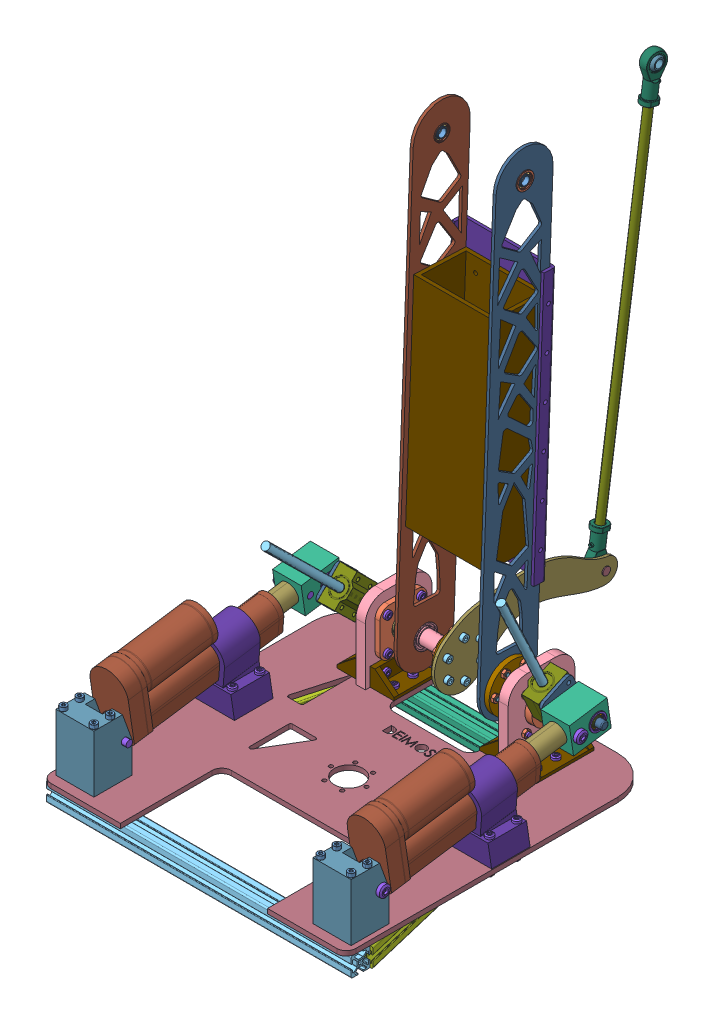
SolidWorks assembly Base + Link1 Final assembly, configuration Default. Lengths in mm.
Overall size (325.65 550.92 510.26).
238 component instances, 41 part files, 304 mates.
Components (placement in the parent):
- linnear rod coupler-1: linnear rod coupler [Default] at (190.8714 137.6403 148.5796) x (0 0.712121 -0.702057) z (-1 0 0) size (18.5 18.5 20.01)
- base bearing assambly-1: base bearing assambly [Default] at (234.6957 114.573 126.7936) x (0 0 1) z (-1 0 0) size (49.5 49.5 22)
  - base shaft bearing housing-1: base shaft bearing housing [Default] at (21.786 23.0673 38.1242) size (49.5 49.5 22)
  - 61802  15x24x5mm-1: 61802  15x24x5mm [Default] at (21.786 23.0673 37.1242) x (0 0 -1) z (1 0 0) size (5 24 24)
  - 61802  15x24x5mm-2: 61802  15x24x5mm [Default] at (21.786 23.0673 22.1242) x (0 0 -1) z (1 0 0) size (5 24 24)
- V8_bearing holder holderURC 2024_V4-1: V8_bearing holder holderURC 2024_V4 [Default] at (213.5714 172.6403 113.5796) x (0 0 1) z (-1 0 0) size (70 80 10)
- linear guid rod-1: linear guid rod [Default] at (184.8714 141.8526 152.8523) x (0.966938 -0.1816 0.179034) z (-0.255013 -0.688576 0.678846) size (8 150 8)
- Connector to Linear bearing-1: Connector to Linear bearing [Default] at (123.1767 129.7873 154.7447) x (1 0 0) z (0 0.553629 0.832764) size (32.2 49.07 49.79)
  - V8_connectorURC 2024_V4-1: V8_connectorURC 2024_V4 [Default] at (40.3948 35.6094 31.6737) x (0 -0.66999 0.74237) z (-1 0 0) size (40 30 30)
  - V8_F688ZZ_assemblyURC 2024_V4-1: V8_F688ZZ_assemblyURC 2024_V4 [Default] at (41.4948 16.099 30.9035) x (0 1 0) z (0 0 1) size (20.89 5 20.89)
    - V8_F688ZZ_shaftURC 2024_V4-1: V8_F688ZZ_shaftURC 2024_V4 [Default] at origin size (10.7 5 10.7)
    - V8_F688ZZ_HousingURC 2024_V4-1: V8_F688ZZ_HousingURC 2024_V4 [Default] x (0.984312 0 0.176438) z (-0.176438 0 0.984312) size (18 5 18)
    - V8_F688ZZ_BallURC 2024_V4-1: V8_F688ZZ_BallURC 2024_V4 [Default] at (5.5752 2.5 -2.1489) x (0.959238 0.232099 0.161224) z (-0.142462 -0.095558 0.985177) size (2 2 2)
    - V8_F688ZZ_BallURC 2024_V4-20: V8_F688ZZ_BallURC 2024_V4 [Default] at (3.2474 2.5 -5.0155) x (0.870805 0.232099 -0.433393) z (0.463818 -0.095558 0.880762) size (2 2 2)
    - V8_F688ZZ_BallURC 2024_V4-21: V8_F688ZZ_BallURC 2024_V4 [Default] at (-0.3209 2.5 -5.9664) x (0.449753 0.232099 -0.862469) z (0.892936 -0.095558 0.439926) size (2 2 2)
    - V8_F688ZZ_BallURC 2024_V4-22: V8_F688ZZ_BallURC 2024_V4 [Default] at (-3.7665 2.5 -4.6383) x (-0.143088 0.232099 -0.96211) z (0.980982 -0.095558 -0.168947) size (2 2 2)
    - V8_F688ZZ_BallURC 2024_V4-23: V8_F688ZZ_BallURC 2024_V4 [Default] at (-5.7735 2.5 -1.5385) x (-0.681275 0.232099 -0.694258) z (0.694326 -0.095558 -0.713288) size (2 2 2)
    - V8_F688ZZ_BallURC 2024_V4-24: V8_F688ZZ_BallURC 2024_V4 [Default] at (-5.5752 2.5 2.1489) x (-0.959238 0.232099 -0.161224) z (0.142462 -0.095558 -0.985177) size (2 2 2)
    - V8_F688ZZ_BallURC 2024_V4-25: V8_F688ZZ_BallURC 2024_V4 [Default] at (-3.2474 2.5 5.0155) x (-0.870805 0.232099 0.433393) z (-0.463818 -0.095558 -0.880762) size (2 2 2)
    - V8_F688ZZ_BallURC 2024_V4-26: V8_F688ZZ_BallURC 2024_V4 [Default] at (0.3209 2.5 5.9664) x (-0.449753 0.232099 0.862469) z (-0.892936 -0.095558 -0.439926) size (2 2 2)
    - V8_F688ZZ_BallURC 2024_V4-27: V8_F688ZZ_BallURC 2024_V4 [Default] at (3.7665 2.5 4.6383) x (0.143088 0.232099 0.96211) z (-0.980982 -0.095558 0.168947) size (2 2 2)
    - V8_F688ZZ_BallURC 2024_V4-28: V8_F688ZZ_BallURC 2024_V4 [Default] at (5.7735 2.5 1.5385) x (0.681275 0.232099 0.694258) z (-0.694326 -0.095558 0.713288) size (2 2 2)
  - V8_F688ZZ_assemblyURC 2024_V4-2: V8_F688ZZ_assemblyURC 2024_V4 [Default] at (9.2948 16.099 30.9035) x (0 -0.381849 0.924225) z (0 0.924225 0.381849) size (20.89 5 20.89)
    - V8_F688ZZ_shaftURC 2024_V4-1: V8_F688ZZ_shaftURC 2024_V4 [Default] at origin size (10.7 5 10.7)
    - V8_F688ZZ_HousingURC 2024_V4-1: V8_F688ZZ_HousingURC 2024_V4 [Default] x (0.984312 0 0.176438) z (-0.176438 0 0.984312) size (18 5 18)
    - V8_F688ZZ_BallURC 2024_V4-1: V8_F688ZZ_BallURC 2024_V4 [Default] at (5.5752 2.5 -2.1489) x (0.959238 0.232099 0.161224) z (-0.142462 -0.095558 0.985177) size (2 2 2)
    - V8_F688ZZ_BallURC 2024_V4-20: V8_F688ZZ_BallURC 2024_V4 [Default] at (3.2474 2.5 -5.0155) x (0.870805 0.232099 -0.433393) z (0.463818 -0.095558 0.880762) size (2 2 2)
    - V8_F688ZZ_BallURC 2024_V4-21: V8_F688ZZ_BallURC 2024_V4 [Default] at (-0.3209 2.5 -5.9664) x (0.449753 0.232099 -0.862469) z (0.892936 -0.095558 0.439926) size (2 2 2)
    - V8_F688ZZ_BallURC 2024_V4-22: V8_F688ZZ_BallURC 2024_V4 [Default] at (-3.7665 2.5 -4.6383) x (-0.143088 0.232099 -0.96211) z (0.980982 -0.095558 -0.168947) size (2 2 2)
    - V8_F688ZZ_BallURC 2024_V4-23: V8_F688ZZ_BallURC 2024_V4 [Default] at (-5.7735 2.5 -1.5385) x (-0.681275 0.232099 -0.694258) z (0.694326 -0.095558 -0.713288) size (2 2 2)
    - V8_F688ZZ_BallURC 2024_V4-24: V8_F688ZZ_BallURC 2024_V4 [Default] at (-5.5752 2.5 2.1489) x (-0.959238 0.232099 -0.161224) z (0.142462 -0.095558 -0.985177) size (2 2 2)
    - V8_F688ZZ_BallURC 2024_V4-25: V8_F688ZZ_BallURC 2024_V4 [Default] at (-3.2474 2.5 5.0155) x (-0.870805 0.232099 0.433393) z (-0.463818 -0.095558 -0.880762) size (2 2 2)
    - V8_F688ZZ_BallURC 2024_V4-26: V8_F688ZZ_BallURC 2024_V4 [Default] at (0.3209 2.5 5.9664) x (-0.449753 0.232099 0.862469) z (-0.892936 -0.095558 -0.439926) size (2 2 2)
    - V8_F688ZZ_BallURC 2024_V4-27: V8_F688ZZ_BallURC 2024_V4 [Default] at (3.7665 2.5 4.6383) x (0.143088 0.232099 0.96211) z (-0.980982 -0.095558 0.168947) size (2 2 2)
    - V8_F688ZZ_BallURC 2024_V4-28: V8_F688ZZ_BallURC 2024_V4 [Default] at (5.7735 2.5 1.5385) x (0.681275 0.232099 0.694258) z (-0.694326 -0.095558 0.713288) size (2 2 2)
- V8_bearing and cam connection_for_v4URC 2024_V4 laser cut-1: V8_bearing and cam connection_for_v4URC 2024_V4 laser cut [Default] at (170.6714 137.31 173.1714) x (0 0.702057 0.712121) z (1 0 0) size (30 35 48)
- V8_LA_Body_V4-1: V8_LA_Body_V4 [Default] at (148.5714 135.8868 383.5572) x (0 -0.989144 -0.146946) z (-1 0 0) size (74 184 40)
- V8_LA_RodURC 2024_V4-1: V8_LA_RodURC 2024_V4 [Default] at (148.5714 158.4515 184.0304) x (1 0 0) z (0 -0.989144 -0.146946) size (20 121 20)
- V8_base plate for LAURC 2024_V4-1: V8_base plate for LAURC 2024_V4 [Default] at (283.5714 87.6403 412.2334) x (0 0 -1) z (0 1 0) size (325 320 5)
- LA_back holder-1: LA_back holder [Default] at (148.5714 152.6403 403.5796) x (-1 0 0) z (0 0 -1) size (40 60 40)
- Connector to Linear bearing-2: Connector to Linear bearing [Default] at (393.1767 131.5103 143.1465) x (1 0 0) z (0 0.553629 0.832764) size (32.2 49.07 49.79)
  - V8_connectorURC 2024_V4-1: V8_connectorURC 2024_V4 [Default] at (40.3948 35.6094 31.6737) x (0 -0.66999 0.74237) z (-1 0 0) size (40 30 30)
  - V8_F688ZZ_assemblyURC 2024_V4-1: V8_F688ZZ_assemblyURC 2024_V4 [Default] at (41.4948 16.099 30.9035) x (0 1 0) z (0 0 1) size (20.89 5 20.89)
    - V8_F688ZZ_shaftURC 2024_V4-1: V8_F688ZZ_shaftURC 2024_V4 [Default] at origin size (10.7 5 10.7)
    - V8_F688ZZ_HousingURC 2024_V4-1: V8_F688ZZ_HousingURC 2024_V4 [Default] x (0.984312 0 0.176438) z (-0.176438 0 0.984312) size (18 5 18)
    - V8_F688ZZ_BallURC 2024_V4-1: V8_F688ZZ_BallURC 2024_V4 [Default] at (5.5752 2.5 -2.1489) x (0.959238 0.232099 0.161224) z (-0.142462 -0.095558 0.985177) size (2 2 2)
    - V8_F688ZZ_BallURC 2024_V4-20: V8_F688ZZ_BallURC 2024_V4 [Default] at (3.2474 2.5 -5.0155) x (0.870805 0.232099 -0.433393) z (0.463818 -0.095558 0.880762) size (2 2 2)
    - V8_F688ZZ_BallURC 2024_V4-21: V8_F688ZZ_BallURC 2024_V4 [Default] at (-0.3209 2.5 -5.9664) x (0.449753 0.232099 -0.862469) z (0.892936 -0.095558 0.439926) size (2 2 2)
    - V8_F688ZZ_BallURC 2024_V4-22: V8_F688ZZ_BallURC 2024_V4 [Default] at (-3.7665 2.5 -4.6383) x (-0.143088 0.232099 -0.96211) z (0.980982 -0.095558 -0.168947) size (2 2 2)
    - V8_F688ZZ_BallURC 2024_V4-23: V8_F688ZZ_BallURC 2024_V4 [Default] at (-5.7735 2.5 -1.5385) x (-0.681275 0.232099 -0.694258) z (0.694326 -0.095558 -0.713288) size (2 2 2)
    - V8_F688ZZ_BallURC 2024_V4-24: V8_F688ZZ_BallURC 2024_V4 [Default] at (-5.5752 2.5 2.1489) x (-0.959238 0.232099 -0.161224) z (0.142462 -0.095558 -0.985177) size (2 2 2)
    - V8_F688ZZ_BallURC 2024_V4-25: V8_F688ZZ_BallURC 2024_V4 [Default] at (-3.2474 2.5 5.0155) x (-0.870805 0.232099 0.433393) z (-0.463818 -0.095558 -0.880762) size (2 2 2)
    - V8_F688ZZ_BallURC 2024_V4-26: V8_F688ZZ_BallURC 2024_V4 [Default] at (0.3209 2.5 5.9664) x (-0.449753 0.232099 0.862469) z (-0.892936 -0.095558 -0.439926) size (2 2 2)
    - V8_F688ZZ_BallURC 2024_V4-27: V8_F688ZZ_BallURC 2024_V4 [Default] at (3.7665 2.5 4.6383) x (0.143088 0.232099 0.96211) z (-0.980982 -0.095558 0.168947) size (2 2 2)
    - V8_F688ZZ_BallURC 2024_V4-28: V8_F688ZZ_BallURC 2024_V4 [Default] at (5.7735 2.5 1.5385) x (0.681275 0.232099 0.694258) z (-0.694326 -0.095558 0.713288) size (2 2 2)
  - V8_F688ZZ_assemblyURC 2024_V4-2: V8_F688ZZ_assemblyURC 2024_V4 [Default] at (9.2948 16.099 30.9035) x (0 -0.381849 0.924225) z (0 0.924225 0.381849) size (20.89 5 20.89)
    - V8_F688ZZ_shaftURC 2024_V4-1: V8_F688ZZ_shaftURC 2024_V4 [Default] at origin size (10.7 5 10.7)
    - V8_F688ZZ_HousingURC 2024_V4-1: V8_F688ZZ_HousingURC 2024_V4 [Default] x (0.984312 0 0.176438) z (-0.176438 0 0.984312) size (18 5 18)
    - V8_F688ZZ_BallURC 2024_V4-1: V8_F688ZZ_BallURC 2024_V4 [Default] at (5.5752 2.5 -2.1489) x (0.959238 0.232099 0.161224) z (-0.142462 -0.095558 0.985177) size (2 2 2)
    - V8_F688ZZ_BallURC 2024_V4-20: V8_F688ZZ_BallURC 2024_V4 [Default] at (3.2474 2.5 -5.0155) x (0.870805 0.232099 -0.433393) z (0.463818 -0.095558 0.880762) size (2 2 2)
    - V8_F688ZZ_BallURC 2024_V4-21: V8_F688ZZ_BallURC 2024_V4 [Default] at (-0.3209 2.5 -5.9664) x (0.449753 0.232099 -0.862469) z (0.892936 -0.095558 0.439926) size (2 2 2)
    - V8_F688ZZ_BallURC 2024_V4-22: V8_F688ZZ_BallURC 2024_V4 [Default] at (-3.7665 2.5 -4.6383) x (-0.143088 0.232099 -0.96211) z (0.980982 -0.095558 -0.168947) size (2 2 2)
    - V8_F688ZZ_BallURC 2024_V4-23: V8_F688ZZ_BallURC 2024_V4 [Default] at (-5.7735 2.5 -1.5385) x (-0.681275 0.232099 -0.694258) z (0.694326 -0.095558 -0.713288) size (2 2 2)
    - V8_F688ZZ_BallURC 2024_V4-24: V8_F688ZZ_BallURC 2024_V4 [Default] at (-5.5752 2.5 2.1489) x (-0.959238 0.232099 -0.161224) z (0.142462 -0.095558 -0.985177) size (2 2 2)
    - V8_F688ZZ_BallURC 2024_V4-25: V8_F688ZZ_BallURC 2024_V4 [Default] at (-3.2474 2.5 5.0155) x (-0.870805 0.232099 0.433393) z (-0.463818 -0.095558 -0.880762) size (2 2 2)
    - V8_F688ZZ_BallURC 2024_V4-26: V8_F688ZZ_BallURC 2024_V4 [Default] at (0.3209 2.5 5.9664) x (-0.449753 0.232099 0.862469) z (-0.892936 -0.095558 -0.439926) size (2 2 2)
    - V8_F688ZZ_BallURC 2024_V4-27: V8_F688ZZ_BallURC 2024_V4 [Default] at (3.7665 2.5 4.6383) x (0.143088 0.232099 0.96211) z (-0.980982 -0.095558 0.168947) size (2 2 2)
    - V8_F688ZZ_BallURC 2024_V4-28: V8_F688ZZ_BallURC 2024_V4 [Default] at (5.7735 2.5 1.5385) x (0.681275 0.232099 0.694258) z (-0.694326 -0.095558 0.713288) size (2 2 2)
- LA_back holder-2: LA_back holder [Default] at (418.5714 152.6403 403.5796) x (-1 0 0) z (0 0 -1) size (40 60 40)
- V8_bearing and cam connection_for_v4URC 2024_V4 laser cut-2: V8_bearing and cam connection_for_v4URC 2024_V4 laser cut [Default] at (396.4714 168.2112 182.1724) x (0 -0.906049 -0.423172) z (-1 0 0) size (30 35 48)
- V8_LA_RodURC 2024_V4-2: V8_LA_RodURC 2024_V4 [Default] at (418.5714 160.1745 172.4322) x (1 0 0) z (0 -0.989144 -0.146946) size (20 121 20)
- linnear rod coupler-2: linnear rod coupler [Default] at (376.2714 137.6403 148.5796) x (0 -0.423172 0.906049) z (1 0 0) size (18.5 18.5 20.01)
- lock_nut_for coupler-2: lock_nut_for coupler [Default] at (396.2714 137.6403 148.5796) x (0 -0.658716 -0.752392) z (1 0 0) size (18 18 13)
- linear guid rod-2: linear guid rod [Default] at (382.2714 133.5883 146.6871) x (0.37331 0.39258 -0.840548) z (0.927707 -0.157974 0.338237) size (8 150 8)
- base bearing assambly-2: base bearing assambly [Default] at (332.4472 114.573 170.3656) x (0 0 -1) z (1 0 0) size (49.5 49.5 22)
  - base shaft bearing housing-1: base shaft bearing housing [Default] at (21.786 23.0673 38.1242) size (49.5 49.5 22)
  - 61802  15x24x5mm-1: 61802  15x24x5mm [Default] at (21.786 23.0673 37.1242) x (0 0 -1) z (1 0 0) size (5 24 24)
  - 61802  15x24x5mm-2: 61802  15x24x5mm [Default] at (21.786 23.0673 22.1242) x (0 0 -1) z (1 0 0) size (5 24 24)
- V8_bearing holder holderURC 2024_V4-2: V8_bearing holder holderURC 2024_V4 [Default] at (353.5714 172.6403 183.5796) x (0 0 -1) z (1 0 0) size (70 80 10)
- V8_LA_Body_V4-2: V8_LA_Body_V4 [Default] at (418.5714 135.8868 383.5572) x (0 -0.989144 -0.146946) z (-1 0 0) size (74 184 40)
- linear bearing robotic arm-1: linear bearing robotic arm [Default] at (182.4393 149.7722 160.8854) x (0 0.712121 -0.702057) z (1 0 0) size (34 30.1 22.2)
- linear bearing robotic arm-2: linear bearing robotic arm [Default] at (384.7035 175.6167 166.3166) x (0 0.423172 -0.906049) z (-1 0 0) size (34 30.1 22.2)
- linear_acutator_holder-1: linear_acutator_holder [Default] at (418.6971 146.656 247.7322) x (0 -0.989144 -0.146946) z (0 -0.146946 0.989144) size (75.87 48 40)
- linear_acutator_holder-2: linear_acutator_holder [Default] at (148.6971 146.656 247.7322) x (0 -0.989144 -0.146946) z (0 -0.146946 0.989144) size (75.87 48 40)
- l bracket_arm base flang-1: l bracket_arm base flang [Default] at (363.5714 111.6403 178.5796) x (0 0 -1) z (1 0 0) size (60 19 25)
- l bracket_arm base flang-2: l bracket_arm base flang [Default] at (353.5714 111.6403 118.5796) x (0 0 1) z (-1 0 0) size (60 19 25)
- l bracket_arm base flang-3: l bracket_arm base flang [Default] at (203.5714 111.6403 118.5796) x (0 0 1) z (-1 0 0) size (60 19 25)
- l bracket_arm base flang-4: l bracket_arm base flang [Default] at (213.5714 111.6403 178.5796) x (0 0 -1) z (1 0 0) size (60 19 25)
- Screw_DIN_912_M4x70_A2.step-1: Screw_DIN_912_M4x70_A2.step [Default] at (402.5714 82.6403 419.5796) size (7 74 7)
- Screw_DIN_912_M4x70_A2.step-2: Screw_DIN_912_M4x70_A2.step [Default] at (434.5714 82.6403 419.5796) x (0.982082 0 -0.188455) z (0.188455 0 0.982082) size (7 74 7)
- Screw_DIN_912_M4x70_A2.step-4: Screw_DIN_912_M4x70_A2.step [Default] at (434.5714 82.6403 402.6026) x (0.918365 0 -0.395734) z (0.395734 0 0.918365) size (7 74 7)
- Screw_DIN_912_M4x70_A2.step-6: Screw_DIN_912_M4x70_A2.step [Default] at (402.5714 82.6403 402.6026) x (0.8 0 -0.6) z (0.6 0 0.8) size (7 74 7)
- Screw_DIN_912_M4x70_A2.step-8: Screw_DIN_912_M4x70_A2.step [Default] at (164.5714 82.6403 419.5796) x (0.63358 0 -0.773678) z (0.773678 0 0.63358) size (7 74 7)
- Screw_DIN_912_M4x70_A2.step-10: Screw_DIN_912_M4x70_A2.step [Default] at (164.5714 82.6403 402.6026) x (0.443629 0 -0.896211) z (0.896211 0 0.443629) size (7 74 7)
- Screw_DIN_912_M4x70_A2.step-12: Screw_DIN_912_M4x70_A2.step [Default] at (132.5714 82.6403 419.5796) x (0.263225 0 -0.964735) z (0.964735 0 0.263225) size (7 74 7)
- Screw_DIN_912_M4x70_A2.step-14: Screw_DIN_912_M4x70_A2.step [Default] at (132.5714 82.6403 402.6026) x (0.120178 0 -0.992752) z (0.992752 0 0.120178) size (7 74 7)
- hex nut style 1 gradeab_iso-8: hex nut style 1 gradeab_iso [ISO - 4032 - M4 - W - N] at (402.5714 84.4403 419.5796) x (0.999814 0 0.019309) z (0 -1 0) size (7 8.08 3.2)
- hex nut style 1 gradeab_iso-9: hex nut style 1 gradeab_iso [ISO - 4032 - M4 - W - N] at (434.5714 84.4403 419.5796) x (0.985538 0 -0.169457) z (0 -1 0) size (7 8.08 3.2)
- hex nut style 1 gradeab_iso-11: hex nut style 1 gradeab_iso [ISO - 4032 - M4 - W - N] at (434.5714 84.4403 402.6026) x (0.563007 0 -0.826452) z (0 -1 0) size (7 8.08 3.2)
- hex nut style 1 gradeab_iso-14: hex nut style 1 gradeab_iso [ISO - 4032 - M4 - W - N] at (402.5714 84.4403 402.6026) x (0.563007 0 -0.826452) z (0 -1 0) size (7 8.08 3.2)
- hex nut style 1 gradeab_iso-16: hex nut style 1 gradeab_iso [ISO - 4032 - M4 - W - N] at (164.5714 84.4403 419.5796) x (0.648401 0 -0.761299) z (0 -1 0) size (7 8.08 3.2)
- hex nut style 1 gradeab_iso-18: hex nut style 1 gradeab_iso [ISO - 4032 - M4 - W - N] at (164.5714 84.4403 402.6026) x (0.563007 0 -0.826452) z (0 -1 0) size (7 8.08 3.2)
- hex nut style 1 gradeab_iso-20: hex nut style 1 gradeab_iso [ISO - 4032 - M4 - W - N] at (132.5714 84.4403 419.5796) x (0.563007 0 -0.826452) z (0 -1 0) size (7 8.08 3.2)
- hex nut style 1 gradeab_iso-22: hex nut style 1 gradeab_iso [ISO - 4032 - M4 - W - N] at (132.5714 84.4403 402.6026) x (0.563007 0 -0.826452) z (0 -1 0) size (7 8.08 3.2)
- V8_shaftURC 2024_V4 real part-1: V8_shaftURC 2024_V4 real part [Default] at (378.5714 128.7575 141.4959) x (-1 0 0) z (0 0.623486 -0.781835) size (75.7 15 15)
- V8_shaftURC 2024_V4-1: V8_shaftURC 2024_V4 [Default] at (223.809 124.5508 145.7858) x (1 0 0) z (0 -0.208738 0.977971) size (115.2 15 15)
- 20 20 aluminium extrusion T slot-1: 20 20 aluminium extrusion T slot [Default] at (4123.5714 77.6403 418.5796) x (0 0 -1) z (-1 0 0) size (20 20 320)
- 20 20 aluminium extrusion T slot 200 mm-1: 20 20 aluminium extrusion T slot 200 mm [Default] at (4183.5714 77.6403 148.5796) x (0 0 -1) z (-1 0 0) size (20 20 200)
- 20 20 aluminium extrusion T slot at angle-1: 20 20 aluminium extrusion T slot at angle [Default] at (-494.3957 77.6403 -3479.2697) x (0.972533 0 -0.232766) z (0.232766 0 0.972533) size (20 20 261.8)
- 20 20 aluminium extrusion T slot at angle-2: 20 20 aluminium extrusion T slot at angle [Default] at (-739.6549 77.6403 4046.3826) x (0.972533 0 0.232766) z (0.232766 0 -0.972533) size (20 20 261.8)
- hexalobular socket pan head_iso-2: hexalobular socket pan head_iso [ISO 14583 - M4 x 12 x 10.6 - 4.8-N] at (378.5714 83.6403 168.5796) size (8 15.1 8)
- hexalobular socket pan head_iso-3: hexalobular socket pan head_iso [ISO 14583 - M4 x 12 x 10.6 - 4.8-N] at (378.5714 83.6403 148.5796) size (8 15.1 8)
- hexalobular socket pan head_iso-4: hexalobular socket pan head_iso [ISO 14583 - M4 x 12 x 10.6 - 4.8-N] at (378.5714 83.6403 128.5796) size (8 15.1 8)
- hexalobular socket pan head_iso-5: hexalobular socket pan head_iso [ISO 14583 - M4 x 12 x 10.6 - 4.8-N] at (338.5714 83.6403 168.5796) size (8 15.1 8)
- hexalobular socket pan head_iso-6: hexalobular socket pan head_iso [ISO 14583 - M4 x 12 x 10.6 - 4.8-N] at (338.5714 83.6403 148.5796) size (8 15.1 8)
- hexalobular socket pan head_iso-7: hexalobular socket pan head_iso [ISO 14583 - M4 x 12 x 10.6 - 4.8-N] at (338.5714 83.6403 128.5796) size (8 15.1 8)
- hexalobular socket pan head_iso-8: hexalobular socket pan head_iso [ISO 14583 - M4 x 12 x 10.6 - 4.8-N] at (228.5714 83.6403 128.5796) size (8 15.1 8)
- hexalobular socket pan head_iso-9: hexalobular socket pan head_iso [ISO 14583 - M4 x 12 x 10.6 - 4.8-N] at (228.5714 83.6403 148.5796) size (8 15.1 8)
- hexalobular socket pan head_iso-10: hexalobular socket pan head_iso [ISO 14583 - M4 x 12 x 10.6 - 4.8-N] at (228.5714 83.6403 168.5796) size (8 15.1 8)
- hexalobular socket pan head_iso-11: hexalobular socket pan head_iso [ISO 14583 - M4 x 12 x 10.6 - 4.8-N] at (188.5714 83.6403 128.5796) size (8 15.1 8)
- hexalobular socket pan head_iso-12: hexalobular socket pan head_iso [ISO 14583 - M4 x 12 x 10.6 - 4.8-N] at (188.5714 83.6403 148.5796) size (8 15.1 8)
- hexalobular socket pan head_iso-13: hexalobular socket pan head_iso [ISO 14583 - M4 x 12 x 10.6 - 4.8-N] at (188.5714 83.6403 168.5796) size (8 15.1 8)
- hexalobular socket pan head_iso-16: hexalobular socket pan head_iso [ISO 14583 - M4 x 25 x 23.6 - 4.8-N] at (373.5714 103.6403 129.5796) x (0 1 0) z (0 0 1) size (8 28.1 8)
- hexalobular socket pan head_iso-17: hexalobular socket pan head_iso [ISO 14583 - M4 x 25 x 23.6 - 4.8-N] at (373.5714 103.6403 148.5796) x (0 1 0) z (0 0 1) size (8 28.1 8)
- hexalobular socket pan head_iso-18: hexalobular socket pan head_iso [ISO 14583 - M4 x 25 x 23.6 - 4.8-N] at (373.5714 103.6403 167.5796) x (0 1 0) z (0 0 1) size (8 28.1 8)
- hexalobular socket pan head_iso-19: hexalobular socket pan head_iso [ISO 14583 - M4 x 25 x 23.6 - 4.8-N] at (193.5714 103.6403 167.5796) x (0 -1 0) z (0 0 1) size (8 28.1 8)
- hexalobular socket pan head_iso-20: hexalobular socket pan head_iso [ISO 14583 - M4 x 25 x 23.6 - 4.8-N] at (193.5714 103.6403 148.5796) x (0 -1 0) z (0 0 1) size (8 28.1 8)
- hexalobular socket pan head_iso-21: hexalobular socket pan head_iso [ISO 14583 - M4 x 25 x 23.6 - 4.8-N] at (193.5714 103.6403 129.5796) x (0 -1 0) z (0 0 1) size (8 28.1 8)
- hexalobular socket pan head_iso-23: hexalobular socket pan head_iso [ISO 14583 - M4 x 20 x 18.6 - 4.8-N] at (368.5714 155.1403 131.0796) x (0 1 0) z (0 0 1) size (8 23.1 8)
- hexalobular socket pan head_iso-24: hexalobular socket pan head_iso [ISO 14583 - M4 x 20 x 18.6 - 4.8-N] at (368.5714 155.1403 166.0796) x (0 1 0) z (0 0 1) size (8 23.1 8)
- hexalobular socket pan head_iso-25: hexalobular socket pan head_iso [ISO 14583 - M4 x 20 x 18.6 - 4.8-N] at (368.5714 120.1403 131.0796) x (0 1 0) z (0 0 1) size (8 23.1 8)
- hexalobular socket pan head_iso-26: hexalobular socket pan head_iso [ISO 14583 - M4 x 20 x 18.6 - 4.8-N] at (368.5714 120.1403 166.0796) x (0 1 0) z (0 0 1) size (8 23.1 8)
- hexalobular socket pan head_iso-27: hexalobular socket pan head_iso [ISO 14583 - M4 x 20 x 18.6 - 4.8-N] at (198.5714 120.1403 131.0796) x (0 -1 0) z (0 0 1) size (8 23.1 8)
- hexalobular socket pan head_iso-28: hexalobular socket pan head_iso [ISO 14583 - M4 x 20 x 18.6 - 4.8-N] at (198.5714 155.1403 131.0796) x (0 -1 0) z (0 0 1) size (8 23.1 8)
- hexalobular socket pan head_iso-29: hexalobular socket pan head_iso [ISO 14583 - M4 x 20 x 18.6 - 4.8-N] at (198.5714 155.1403 166.0796) x (0 -1 0) z (0 0 1) size (8 23.1 8)
- hexalobular socket pan head_iso-30: hexalobular socket pan head_iso [ISO 14583 - M4 x 20 x 18.6 - 4.8-N] at (198.5714 120.1403 166.0796) x (0 -1 0) z (0 0 1) size (8 23.1 8)
- hexalobular socket pan head_iso-32: hexalobular socket pan head_iso [ISO 14583 - M4 x 35 x 33.6 - 4.8-N] at (437.6971 83.0703 277.3153) size (8 38.1 8)
- hexalobular socket pan head_iso-33: hexalobular socket pan head_iso [ISO 14583 - M4 x 35 x 33.6 - 4.8-N] at (437.6971 83.0703 248.7068) size (8 38.1 8)
- hexalobular socket pan head_iso-34: hexalobular socket pan head_iso [ISO 14583 - M4 x 35 x 33.6 - 4.8-N] at (399.6971 83.0703 277.3153) size (8 38.1 8)
- hexalobular socket pan head_iso-35: hexalobular socket pan head_iso [ISO 14583 - M4 x 35 x 33.6 - 4.8-N] at (399.6971 83.0703 248.7068) size (8 38.1 8)
- hexalobular socket pan head_iso-36: hexalobular socket pan head_iso [ISO 14583 - M4 x 35 x 33.6 - 4.8-N] at (129.6971 83.0703 248.7068) size (8 38.1 8)
- hexalobular socket pan head_iso-37: hexalobular socket pan head_iso [ISO 14583 - M4 x 35 x 33.6 - 4.8-N] at (129.6971 83.0703 277.3153) size (8 38.1 8)
- hexalobular socket pan head_iso-38: hexalobular socket pan head_iso [ISO 14583 - M4 x 35 x 33.6 - 4.8-N] at (167.6971 83.0703 248.7068) size (8 38.1 8)
- hexalobular socket pan head_iso-39: hexalobular socket pan head_iso [ISO 14583 - M4 x 35 x 33.6 - 4.8-N] at (167.6971 83.0703 277.3153) size (8 38.1 8)
- hexalobular socket pan head_iso-41: hexalobular socket pan head_iso [ISO 14583 - M6 x 30 x 28 - 4.8-N] at (163.5714 157.4228 190.9544) x (0 1 0) z (0 0 1) size (12 34.6 12)
- hexalobular socket pan head_iso-42: hexalobular socket pan head_iso [ISO 14583 - M6 x 30 x 28 - 4.8-N] at (403.5714 159.1459 179.3562) x (0 -1 0) z (0 0 1) size (12 34.6 12)
- hex nut style 1 gradeab_iso-24: hex nut style 1 gradeab_iso [ISO - 4032 - M4 - W - N] at (371.7714 103.6403 148.5796) x (0 0.916221 0.400674) z (1 0 0) size (7 8.08 3.2)
- hex nut style 1 gradeab_iso-25: hex nut style 1 gradeab_iso [ISO - 4032 - M4 - W - N] at (371.7714 103.6403 167.5796) x (0 0 -1) z (1 0 0) size (7 8.08 3.2)
- hex nut style 1 gradeab_iso-26: hex nut style 1 gradeab_iso [ISO - 4032 - M4 - W - N] at (371.7714 103.6403 129.5796) x (0 0 -1) z (1 0 0) size (7 8.08 3.2)
- hex nut style 1 gradeab_iso-27: hex nut style 1 gradeab_iso [ISO - 4032 - M4 - W - N] at (366.7714 120.1403 131.0796) x (0 0 -1) z (1 0 0) size (7 8.08 3.2)
- hex nut style 1 gradeab_iso-28: hex nut style 1 gradeab_iso [ISO - 4032 - M4 - W - N] at (366.7714 155.1403 131.0796) x (0 0.719892 -0.694086) z (1 0 0) size (7 8.08 3.2)
- hex nut style 1 gradeab_iso-29: hex nut style 1 gradeab_iso [ISO - 4032 - M4 - W - N] at (366.7714 155.1403 166.0796) x (0 0 -1) z (1 0 0) size (7 8.08 3.2)
- hex nut style 1 gradeab_iso-30: hex nut style 1 gradeab_iso [ISO - 4032 - M4 - W - N] at (378.5714 84.4403 128.5796) x (1 0 0) z (0 -1 0) size (7 8.08 3.2)
- hex nut style 1 gradeab_iso-31: hex nut style 1 gradeab_iso [ISO - 4032 - M4 - W - N] at (338.5714 84.4403 128.5796) x (1 0 0) z (0 -1 0) size (7 8.08 3.2)
- hex nut style 1 gradeab_iso-32: hex nut style 1 gradeab_iso [ISO - 4032 - M4 - W - N] at (338.5714 84.4403 168.5796) x (1 0 0) z (0 -1 0) size (7 8.08 3.2)
- hex nut style 1 gradeab_iso-34: hex nut style 1 gradeab_iso [ISO - 4032 - M4 - W - N] at (366.7714 120.1403 166.0796) x (0 0 -1) z (1 0 0) size (7 8.08 3.2)
- hex nut style 1 gradeab_iso-35: hex nut style 1 gradeab_iso [ISO - 4032 - M4 - W - N] at (200.3714 155.1403 131.0796) x (0 0 1) z (-1 0 0) size (7 8.08 3.2)
- hex nut style 1 gradeab_iso-36: hex nut style 1 gradeab_iso [ISO - 4032 - M4 - W - N] at (200.3714 120.1403 131.0796) x (0 0 1) z (-1 0 0) size (7 8.08 3.2)
- hex nut style 1 gradeab_iso-37: hex nut style 1 gradeab_iso [ISO - 4032 - M4 - W - N] at (200.3714 155.1403 166.0796) x (0 0 1) z (-1 0 0) size (7 8.08 3.2)
- hex nut style 1 gradeab_iso-38: hex nut style 1 gradeab_iso [ISO - 4032 - M4 - W - N] at (200.3714 120.1403 166.0796) x (0 0 1) z (-1 0 0) size (7 8.08 3.2)
- hex nut style 1 gradeab_iso-39: hex nut style 1 gradeab_iso [ISO - 4032 - M4 - W - N] at (195.3714 103.6403 148.5796) x (0 0 1) z (-1 0 0) size (7 8.08 3.2)
- hex nut style 1 gradeab_iso-40: hex nut style 1 gradeab_iso [ISO - 4032 - M4 - W - N] at (195.3714 103.6403 167.5796) x (0 0 1) z (-1 0 0) size (7 8.08 3.2)
- hex nut style 1 gradeab_iso-41: hex nut style 1 gradeab_iso [ISO - 4032 - M4 - W - N] at (195.3714 103.6403 129.5796) x (0 0 1) z (-1 0 0) size (7 8.08 3.2)
- hex nut style 1 gradeab_iso-42: hex nut style 1 gradeab_iso [ISO - 4032 - M4 - W - N] at (228.5714 84.4403 128.5796) x (1 0 0) z (0 -1 0) size (7 8.08 3.2)
- hex nut style 1 gradeab_iso-43: hex nut style 1 gradeab_iso [ISO - 4032 - M4 - W - N] at (188.5714 84.4403 128.5796) x (1 0 0) z (0 -1 0) size (7 8.08 3.2)
- hex nut style 1 gradeab_iso-44: hex nut style 1 gradeab_iso [ISO - 4032 - M4 - W - N] at (228.5714 84.4403 168.5796) x (1 0 0) z (0 -1 0) size (7 8.08 3.2)
- hex nut style 1 gradeab_iso-45: hex nut style 1 gradeab_iso [ISO - 4032 - M4 - W - N] at (129.6971 84.4403 277.3153) x (1 0 0) z (0 -1 0) size (7 8.08 3.2)
- hex nut style 1 gradeab_iso-46: hex nut style 1 gradeab_iso [ISO - 4032 - M4 - W - N] at (129.6971 84.4403 248.7068) x (1 0 0) z (0 -1 0) size (7 8.08 3.2)
- hex nut style 1 gradeab_iso-47: hex nut style 1 gradeab_iso [ISO - 4032 - M4 - W - N] at (437.6971 84.4403 277.3153) x (-0.32211 0 -0.946702) z (0 -1 0) size (7 8.08 3.2)
- hex nut style 1 gradeab_iso-48: hex nut style 1 gradeab_iso [ISO - 4032 - M4 - W - N] at (437.4458 84.4403 248.7068) x (0.082905 0 -0.996557) z (0 -1 0) size (7 8.08 3.2)
- hexalobular socket pan head_iso-44: hexalobular socket pan head_iso [ISO 14583 - M6 x 45 x 38 - 4.8-N] at (173.5714 127.6403 391.4309) x (0 1 0) z (0 0 1) size (12 49.6 12)
- hexalobular socket pan head_iso-45: hexalobular socket pan head_iso [ISO 14583 - M6 x 45 x 43 - 4.8-N] at (393.5714 127.6403 391.4309) x (0 -1 0) z (0 0 1) size (12 49.6 12)
- Base Shaft connector to link 1-1: Base Shaft connector to link 1 [Default] at (328.5714 137.6403 148.5796) x (0 -0.999275 0.038083) z (1 0 0) size (50 50 15)
- lock_nut_for coupler-3: lock_nut_for coupler [Default] at (170.8714 137.6403 148.5796) x (0 0.443849 0.896102) z (-1 0 0) size (18 18 13)
- Base Shaft connector to link 1-2: Base Shaft connector to link 1 [Default] at (278.0714 137.6403 148.5796) x (0 -0.031224 0.999512) z (-1 0 0) size (50 50 15)
- Link 1 assmebly-1: Link 1 assmebly [Default] at (819.6937 160.5949 424.8752) x (0 0.999275 -0.038083) z (-1 0 0) size (512.01 240.32 96.64)
  - V8_link 1_real_transmisionURC 2024-1: V8_link 1_real_transmisionURC 2024 [Default] at (-12.4157 276.9693 491.1223) size (510 60 3)
  - V8_link 1_fack_transmisionURC 2024-1: V8_link 1_fack_transmisionURC 2024 [Default] at (-12.4157 276.9693 581.1223) x (1 0 0) z (0 0 -1) size (510 60 3)
  - V8_link_2_power_rod_1_v4URC 2024-1: V8_link_2_power_rod_1_v4URC 2024 [Default] at (-12.4157 276.9693 541.6223) x (0.069266 0.997598 0) z (0 0 -1) size (192.5 77 3)
  - connecting rod link 2 lower shaft-1: connecting rod link 2 lower shaft [Default] at (-2.0258 426.6091 537.6223) x (0.99828 -0.058626 0) z (0 0 1) size (8 8 20)
  - V8_ball with 8mm holeURC 2024-1: V8_ball with 8mm holeURC 2024 [Default] at (-2.0258 426.6091 543.6223) x (0.927927 0.372761 0) z (0.372761 -0.927927 0) size (15.88 12 15.88)
  - V8_Ball mounting partURC 2024-1: V8_Ball mounting partURC 2024 [Default] at (33.7808 430.3417 549.6223) x (0.103588 -0.99462 0) z (0.99462 0.103588 0) size (22 14 47)
  - power connecting rod-1: power connecting rod [Default] at (411.7365 469.7053 549.6223) x (0.084556 -0.811876 -0.577674) z (-0.05984 0.574566 -0.816268) size (8 400 8)
  - V8_link_1 coverURC 2024-1: V8_link_1 coverURC 2024 [Default] at (347.5286 412.1474 584.1223) x (-1 0 0) z (0 0 -1) size (280 12.82 96.64)
  - V8_electronics box of robotic armURC 2024-1: V8_electronics box of robotic armURC 2024 [Default] at (322.236 306.9693 578.1223) x (-1 0 0) z (0 0 -1) size (225 55 84)
  - V8_Ball mounting partURC 2024-2: V8_Ball mounting partURC 2024 [Default] at (391.8441 467.6335 549.6223) x (-0.103034 0.989295 -0.103341) z (-0.99462 -0.103588 0) size (22 14 47)
  - V8_ball with 8mm holeURC 2024-2: V8_ball with 8mm holeURC 2024 [Default] at (427.6538 471.3623 543.6223) x (1 0 0) z (0 -1 0) size (15.88 12 15.88)
  - V8_F688ZZ_assemblyURC 2024-1: V8_F688ZZ_assemblyURC 2024 [Default] at (437.5843 276.9693 490.0223) x (1 0 0) z (0 -1 0) size (20.89 5 20.89)
    - V8_F688ZZ_shaftURC 2024-1: V8_F688ZZ_shaftURC 2024 [Default] at origin size (10.7 5 10.7)
    - V8_F688ZZ_HousingURC 2024-1: V8_F688ZZ_HousingURC 2024 [Default] x (0.984312 0 0.176438) z (-0.176438 0 0.984312) size (18 5 18)
    - V8_F688ZZ_BallURC 2024-1: V8_F688ZZ_BallURC 2024 [Default] at (5.5752 2.5 -2.1489) x (0.959238 0.232099 0.161224) z (-0.142462 -0.095558 0.985177) size (2 2 2)
    - V8_F688ZZ_BallURC 2024-20: V8_F688ZZ_BallURC 2024 [Default] at (3.2474 2.5 -5.0155) x (0.870805 0.232099 -0.433393) z (0.463818 -0.095558 0.880762) size (2 2 2)
    - V8_F688ZZ_BallURC 2024-21: V8_F688ZZ_BallURC 2024 [Default] at (-0.3209 2.5 -5.9664) x (0.449753 0.232099 -0.862469) z (0.892936 -0.095558 0.439926) size (2 2 2)
    - V8_F688ZZ_BallURC 2024-22: V8_F688ZZ_BallURC 2024 [Default] at (-3.7665 2.5 -4.6383) x (-0.143088 0.232099 -0.96211) z (0.980982 -0.095558 -0.168947) size (2 2 2)
    - V8_F688ZZ_BallURC 2024-23: V8_F688ZZ_BallURC 2024 [Default] at (-5.7735 2.5 -1.5385) x (-0.681275 0.232099 -0.694258) z (0.694326 -0.095558 -0.713288) size (2 2 2)
    - V8_F688ZZ_BallURC 2024-24: V8_F688ZZ_BallURC 2024 [Default] at (-5.5752 2.5 2.1489) x (-0.959238 0.232099 -0.161224) z (0.142462 -0.095558 -0.985177) size (2 2 2)
    - V8_F688ZZ_BallURC 2024-25: V8_F688ZZ_BallURC 2024 [Default] at (-3.2474 2.5 5.0155) x (-0.870805 0.232099 0.433393) z (-0.463818 -0.095558 -0.880762) size (2 2 2)
    - V8_F688ZZ_BallURC 2024-26: V8_F688ZZ_BallURC 2024 [Default] at (0.3209 2.5 5.9664) x (-0.449753 0.232099 0.862469) z (-0.892936 -0.095558 -0.439926) size (2 2 2)
    - V8_F688ZZ_BallURC 2024-27: V8_F688ZZ_BallURC 2024 [Default] at (3.7665 2.5 4.6383) x (0.143088 0.232099 0.96211) z (-0.980982 -0.095558 0.168947) size (2 2 2)
    - V8_F688ZZ_BallURC 2024-28: V8_F688ZZ_BallURC 2024 [Default] at (5.7735 2.5 1.5385) x (0.681275 0.232099 0.694258) z (-0.694326 -0.095558 0.713288) size (2 2 2)
  - V8_F688ZZ_assemblyURC 2024-2: V8_F688ZZ_assemblyURC 2024 [Default] at (437.5843 276.9693 582.2223) x (1 0.000487 0) z (-0.000487 1 0) size (20.89 5 20.89)
    - V8_F688ZZ_shaftURC 2024-1: V8_F688ZZ_shaftURC 2024 [Default] at origin size (10.7 5 10.7)
    - V8_F688ZZ_HousingURC 2024-1: V8_F688ZZ_HousingURC 2024 [Default] x (0.984312 0 0.176438) z (-0.176438 0 0.984312) size (18 5 18)
    - V8_F688ZZ_BallURC 2024-1: V8_F688ZZ_BallURC 2024 [Default] at (5.5752 2.5 -2.1489) x (0.959238 0.232099 0.161224) z (-0.142462 -0.095558 0.985177) size (2 2 2)
    - V8_F688ZZ_BallURC 2024-20: V8_F688ZZ_BallURC 2024 [Default] at (3.2474 2.5 -5.0155) x (0.870805 0.232099 -0.433393) z (0.463818 -0.095558 0.880762) size (2 2 2)
    - V8_F688ZZ_BallURC 2024-21: V8_F688ZZ_BallURC 2024 [Default] at (-0.3209 2.5 -5.9664) x (0.449753 0.232099 -0.862469) z (0.892936 -0.095558 0.439926) size (2 2 2)
    - V8_F688ZZ_BallURC 2024-22: V8_F688ZZ_BallURC 2024 [Default] at (-3.7665 2.5 -4.6383) x (-0.143088 0.232099 -0.96211) z (0.980982 -0.095558 -0.168947) size (2 2 2)
    - V8_F688ZZ_BallURC 2024-23: V8_F688ZZ_BallURC 2024 [Default] at (-5.7735 2.5 -1.5385) x (-0.681275 0.232099 -0.694258) z (0.694326 -0.095558 -0.713288) size (2 2 2)
    - V8_F688ZZ_BallURC 2024-24: V8_F688ZZ_BallURC 2024 [Default] at (-5.5752 2.5 2.1489) x (-0.959238 0.232099 -0.161224) z (0.142462 -0.095558 -0.985177) size (2 2 2)
    - V8_F688ZZ_BallURC 2024-25: V8_F688ZZ_BallURC 2024 [Default] at (-3.2474 2.5 5.0155) x (-0.870805 0.232099 0.433393) z (-0.463818 -0.095558 -0.880762) size (2 2 2)
    - V8_F688ZZ_BallURC 2024-26: V8_F688ZZ_BallURC 2024 [Default] at (0.3209 2.5 5.9664) x (-0.449753 0.232099 0.862469) z (-0.892936 -0.095558 -0.439926) size (2 2 2)
    - V8_F688ZZ_BallURC 2024-27: V8_F688ZZ_BallURC 2024 [Default] at (3.7665 2.5 4.6383) x (0.143088 0.232099 0.96211) z (-0.980982 -0.095558 0.168947) size (2 2 2)
    - V8_F688ZZ_BallURC 2024-28: V8_F688ZZ_BallURC 2024 [Default] at (5.7735 2.5 1.5385) x (0.681275 0.232099 0.694258) z (-0.694326 -0.095558 0.713288) size (2 2 2)
- radial ball bearing_68_iso-1: radial ball bearing_68_iso [ISO 15 RBB - 1815 - 18,SI,NC,18_68] at (240.0714 137.6403 148.5796) size (5 24 24)
- socket head cap screw_iso-2: socket head cap screw_iso [ISO 4762 M4 x 12 - 12N] at (321.5714 154.5674 137.9272) size (16 7 7)
- socket head cap screw_iso-3: socket head cap screw_iso [ISO 4762 M4 x 12 - 12N] at (321.5714 155.329 157.9127) size (16 7 7)
- socket head cap screw_iso-4: socket head cap screw_iso [ISO 4762 M4 x 12 - 12N] at (321.5714 138.4019 168.5651) size (16 7 7)
- socket head cap screw_iso-5: socket head cap screw_iso [ISO 4762 M4 x 12 - 12N] at (321.5714 120.7132 159.232) size (16 7 7)
- socket head cap screw_iso-6: socket head cap screw_iso [ISO 4762 M4 x 12 - 12N] at (321.5714 119.9515 139.2465) size (16 7 7)
- socket head cap screw_iso-7: socket head cap screw_iso [ISO 4762 M4 x 12 - 12N] at (321.5714 136.8786 128.5941) size (16 7 7)
- socket head cap screw_iso-8: socket head cap screw_iso [ISO 4762 M4 x 12 - 12N] at (285.0714 157.6305 149.2041) x (-1 0 0) z (0 0.924225 0.381849) size (16 7 7)
- socket head cap screw_iso-9: socket head cap screw_iso [ISO 4762 M4 x 12 - 12N] at (285.0714 148.1762 131.5798) x (-1 0 0) z (0 0.924225 0.381849) size (16 7 7)
- socket head cap screw_iso-10: socket head cap screw_iso [ISO 4762 M4 x 12 - 12N] at (285.0714 128.186 130.9553) x (-1 0 0) z (0 0.924225 0.381849) size (16 7 7)
- socket head cap screw_iso-11: socket head cap screw_iso [ISO 4762 M4 x 12 - 12N] at (285.0714 117.65 147.9551) x (-1 0 0) z (0 0.924225 0.381849) size (16 7 7)
- socket head cap screw_iso-12: socket head cap screw_iso [ISO 4762 M4 x 12 - 12N] at (285.0714 127.1043 165.5794) x (-1 0 0) z (0 0.924225 0.381849) size (16 7 7)
